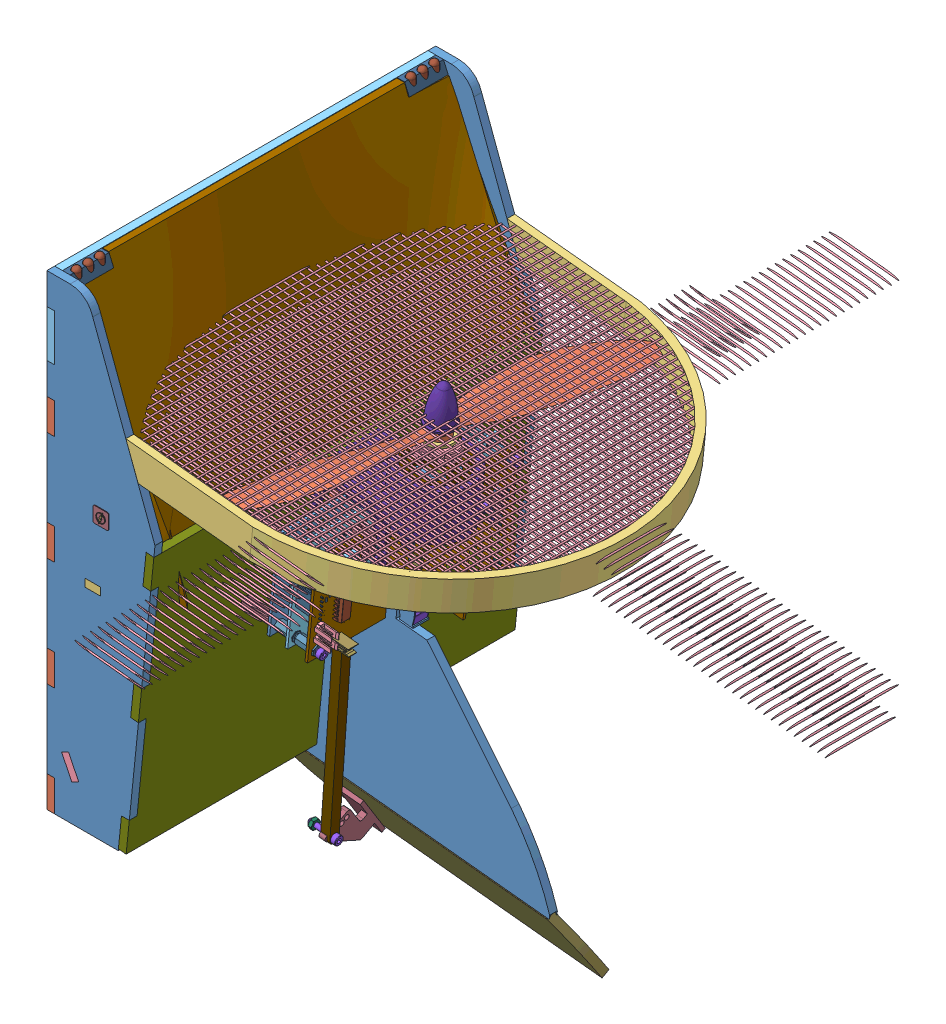
SolidWorks assembly AssTotaleSimu2, configuration Défaut. Lengths in mm. (continued)
Components (placement in the parent): (continued)
- AssStructSimu-1: AssStructSimu [Défaut] at (-125.7658 -1.8483 624.6548) x (1 0 0) z (0 0 -1) size (253.25 324.59 251.6) (continued)
  - AssCarte-1: AssCarte [Défaut] at (38.0121 147.1029 290.772) x (-0.101852 0.9948 0) z (0.9948 0.101852 0) size (66.52 130.57 98.72) (continued)
    - AssEntretoise-3: AssEntretoise [Défaut] at (-106.8199 -51.2976 37.1344) x (0 0 -1) z (1 0 0) size (58.24 7.29 7.81)
      - socket head cap screw 4762_din-1: socket head cap screw 4762_din [EN ISO 4762 M3 x 5 - 5N] at (-2.4967 0.5867 0) size (8 5.5 5.5)
      - hexagonal_spacer_MF_M3_H20_HEX5.5_FTD6_MTL6-1: hexagonal_spacer_MF_M3_H20_HEX5.5_FTD6_MTL6 [Défaut] at (48.3433 0.5867 0) x (0 0 1) z (-1 0 0) size (6.36 5.51 26)
      - hex nut style 1 gradeab_din-1: hex nut style 1 gradeab_din [Hexagon Nut ISO 4032 - M3 - W - N] at (53.3433 0.5867 0) x (0 0.943962 0.330053) z (-1 0 0) size (5.5 6.35 2.4)
      - hexagonal_spacer_MF_M3_H12_HEX5.5_FTD6_MTL6-2: hexagonal_spacer_MF_M3_H12_HEX5.5_FTD6_MTL6 [Défaut] at (27.0633 0.5867 0) x (0 0.248308 0.968681) z (-1 0 0) size (6.36 5.51 18)
      - hexagonal_spacer_MF_M3_H12_HEX5.5_FTD6_MTL6-3: hexagonal_spacer_MF_M3_H12_HEX5.5_FTD6_MTL6 [Défaut] at (13.7833 0.5867 0) x (0 0 1) z (-1 0 0) size (6.36 5.51 18)
    - AssEntretoise-4: AssEntretoise [Défaut] at (-106.8199 68.7024 37.1344) x (0 0 -1) z (1 0 0) size (58.24 7.29 7.81)
      - socket head cap screw 4762_din-1: socket head cap screw 4762_din [EN ISO 4762 M3 x 5 - 5N] at (-2.4967 0.5867 0) size (8 5.5 5.5)
      - hexagonal_spacer_MF_M3_H20_HEX5.5_FTD6_MTL6-1: hexagonal_spacer_MF_M3_H20_HEX5.5_FTD6_MTL6 [Défaut] at (48.3433 0.5867 0) x (0 0 1) z (-1 0 0) size (6.36 5.51 26)
      - hex nut style 1 gradeab_din-1: hex nut style 1 gradeab_din [Hexagon Nut ISO 4032 - M3 - W - N] at (53.3433 0.5867 0) x (0 0.943962 0.330053) z (-1 0 0) size (5.5 6.35 2.4)
      - hexagonal_spacer_MF_M3_H12_HEX5.5_FTD6_MTL6-2: hexagonal_spacer_MF_M3_H12_HEX5.5_FTD6_MTL6 [Défaut] at (27.0633 0.5867 0) x (0 0.248308 0.968681) z (-1 0 0) size (6.36 5.51 18)
      - hexagonal_spacer_MF_M3_H12_HEX5.5_FTD6_MTL6-3: hexagonal_spacer_MF_M3_H12_HEX5.5_FTD6_MTL6 [Défaut] at (13.7833 0.5867 0) x (0 0 1) z (-1 0 0) size (6.36 5.51 18)
    - AssMpu-1: AssMpu [Défaut] at (-150.6881 40.5798 29.6372) x (0.908747 0.417347 0) z (0 0 1) size (8 8 22.28)
      - hex nut style 1 gradeab_din-1: hex nut style 1 gradeab_din [Hexagon Nut ISO 4032 - M3 - W - N] at (0.2783 0.3227 1.2) size (5.5 6.35 2.4)
      - plain washer 6903 type ab_din-1: plain washer 6903 type ab_din [DIN 6903-A3] at (0.2783 0.3227 1.2) x (0 0 1) z (-1 0 0) size (1 8 8)
      - socket head cap screw 4762_din-1: socket head cap screw 4762_din [EN ISO 4762 M3 x 5 - 5N] at (0.2783 0.3227 19.76) x (0 0 -1) z (-0.852155 0.523289 0) size (8 5.5 5.5)
      - hexagonal_spacer_MF_M3_H12_HEX5.5_FTD6_MTL6-1: hexagonal_spacer_MF_M3_H12_HEX5.5_FTD6_MTL6 [Défaut] at (0.2783 0.3227 3.48) size (6.36 5.51 18)
    - AssMpu-2: AssMpu [Défaut] at (-130.3481 40.6665 29.6372) size (8 8 22.28)
      - hex nut style 1 gradeab_din-1: hex nut style 1 gradeab_din [Hexagon Nut ISO 4032 - M3 - W - N] at (0.2783 0.3227 1.2) size (5.5 6.35 2.4)
      - plain washer 6903 type ab_din-1: plain washer 6903 type ab_din [DIN 6903-A3] at (0.2783 0.3227 1.2) x (0 0 1) z (-1 0 0) size (1 8 8)
      - socket head cap screw 4762_din-1: socket head cap screw 4762_din [EN ISO 4762 M3 x 5 - 5N] at (0.2783 0.3227 19.76) x (0 0 -1) z (-0.852155 0.523289 0) size (8 5.5 5.5)
      - hexagonal_spacer_MF_M3_H12_HEX5.5_FTD6_MTL6-1: hexagonal_spacer_MF_M3_H12_HEX5.5_FTD6_MTL6 [Défaut] at (0.2783 0.3227 3.48) size (6.36 5.51 18)
    - AssCosse-1: AssCosse [Défaut] at (-142.6764 26.8797 71.168) x (0 -1 0) z (-0.344896 0 -0.938641) size (9.83 18.66 11.64)
      - socket head cap screw 4762_din-1: socket head cap screw 4762_din [EN ISO 4762 M3 x 6 - 6N] at (-5.1064 0.3659 0) size (9 5.5 5.5)
      - plain washer 6903 type ab_din-1: plain washer 6903 type ab_din [DIN 6903-A3] at (-2.1064 0.3659 0) size (1 8 8)
      - hex nut style 1 gradeab_din-2: hex nut style 1 gradeab_din [Hexagon Nut ISO 4032 - M3 - W - N] at (1.281 0.3659 0) x (0 0.924225 0.381849) z (-1 0 0) size (5.5 6.35 2.4)
      - 31880-1: 31880 [Default] at (0.4936 0.3659 0) x (0 0.344896 -0.938641) z (0 -0.938641 -0.344896) size (5.54 5 17.37)
    - AssCosse-2: AssCosse [Défaut] at (-142.6764 -2.9203 71.168) x (0 -1 0) z (-0.344896 0 -0.938641) size (9.83 18.66 11.64)
      - socket head cap screw 4762_din-1: socket head cap screw 4762_din [EN ISO 4762 M3 x 6 - 6N] at (-5.1064 0.3659 0) size (9 5.5 5.5)
      - plain washer 6903 type ab_din-1: plain washer 6903 type ab_din [DIN 6903-A3] at (-2.1064 0.3659 0) size (1 8 8)
      - hex nut style 1 gradeab_din-2: hex nut style 1 gradeab_din [Hexagon Nut ISO 4032 - M3 - W - N] at (1.281 0.3659 0) x (0 0.924225 0.381849) z (-1 0 0) size (5.5 6.35 2.4)
      - 31880-1: 31880 [Default] at (0.4936 0.3659 0) x (0 0.344896 -0.938641) z (0 -0.938641 -0.344896) size (5.54 5 17.37)
    - AssCosse-3: AssCosse [Défaut] at (-142.6764 12.0797 71.168) x (0 -1 0) z (-0.344896 0 -0.938641) size (9.83 18.66 11.64)
      - socket head cap screw 4762_din-1: socket head cap screw 4762_din [EN ISO 4762 M3 x 6 - 6N] at (-5.1064 0.3659 0) size (9 5.5 5.5)
      - plain washer 6903 type ab_din-1: plain washer 6903 type ab_din [DIN 6903-A3] at (-2.1064 0.3659 0) size (1 8 8)
      - hex nut style 1 gradeab_din-2: hex nut style 1 gradeab_din [Hexagon Nut ISO 4032 - M3 - W - N] at (1.281 0.3659 0) x (0 0.924225 0.381849) z (-1 0 0) size (5.5 6.35 2.4)
      - 31880-1: 31880 [Default] at (0.4936 0.3659 0) x (0 0.344896 -0.938641) z (0 -0.938641 -0.344896) size (5.54 5 17.37)
    - Terminal_QD_Female-1: Terminal_QD_Female [Default] at (-137.2199 31.5422 53.3942) x (0 1 0) z (-1 0 0) size (9.4 5.5 22.35)
    - Terminal_QD_Female-2: Terminal_QD_Female [Default] at (-137.3199 31.5422 36.2942) x (0 -1 0) z (-1 0 0) size (9.4 5.5 22.35)
    - Terminal_QD_Female-3: Terminal_QD_Female [Default] at (-137.2199 1.7422 53.3942) x (0 1 0) z (-1 0 0) size (9.4 5.5 22.35)
    - Terminal_QD_Female-4: Terminal_QD_Female [Default] at (-137.3199 1.7422 35.9942) x (0 1 0) z (-1 0 0) size (9.4 5.5 22.35)
    - Terminal_QD_Female-5: Terminal_QD_Female [Default] at (-137.3199 16.7422 35.9942) x (0 1 0) z (-1 0 0) size (9.4 5.5 22.35)
    - Terminal_QD_Female-6: Terminal_QD_Female [Default] at (-137.2199 16.7422 53.3942) x (0 1 0) z (-1 0 0) size (9.4 5.5 22.35)
- AssTige-1: AssTige [Défaut] at (-241.576 -121.7726 340.4233) x (-0.101791 -0.994204 -0.034587) z (0.9948 -0.101852 0) size (166.39 7.19 19)
  - tige_servo-1: tige_servo [Défaut] at (-106.2712 0.2685 162) size (165 6 6)
  - socket head cap screw 4762_din-2: socket head cap screw 4762_din [EN ISO 4762 M2 x 10 - 10N] at (-104.2712 3.2685 170) x (0 0 -1) z (0.923728 0.383049 0) size (12 3.8 3.8)
  - hex nut style 1 gradeab_din-1: hex nut style 1 gradeab_din [Hexagon Nut ISO 4032 - M3 - W - N] at (55.7288 3.2685 156) size (5.5 6.35 2.4)
  - hex nut style 1 gradeab_din-2: hex nut style 1 gradeab_din [Hexagon Nut ISO 4032 - M2 - W - N] at (-104.2712 3.2685 160) x (0.904801 0.425836 0) z (0 0 1) size (4 4.62 1.6)
  - socket head cap screw 4762_din-3: socket head cap screw 4762_din [EN ISO 4762 M3 x 16 - 16N] at (55.7288 3.2685 171) x (0 0 -1) z (0.923728 0.383049 0) size (19 5.5 5.5)
- AssGoPro-1: AssGoPro [Défaut] at (-119.9926 15.1708 318.2917) x (0 0 -1) z (-0.119031 -0.99289 0) size (64.3 52.3 34.42)
  - GoPRo Frame for LCD Screen-1: GoPRo Frame for LCD Screen [Défaut] at (-2.6935 10.9558 5.5635) size (64.3 47.42 34.42)
    - GoProFrame MJM-1: GoProFrame MJM [Défaut] at (-3.6084 -1.6692 52.45) size (64.3 59.3 23.5)
    - GoPro Hero 3 Front Panel-1: GoPro Hero 3 Front Panel [Défaut] at (-3.6084 -1.6692 55.7) x (-1 0 0) z (0 0 -1) size (59.25 41.2 1.9)
    - GoPro Hero 3 Screen-1: GoPro Hero 3 Screen [Défaut] at (12.7166 3.9308 54.9) size (15 18 1)
    - GoPro Hero 3 Mode Button-1: GoPro Hero 3 Mode Button [Défaut] at (13.4166 -12.4692 54.95) x (-1 0 0) z (0 0 -1) size (11.97 12.11 3.03)
    - GoPro Hero 3 LED Cover-1: GoPro Hero 3 LED Cover [Défaut] at (3.1166 -9.3192 54.85) x (-0.999988 0.004848 0) z (0 0 -1) size (5 5 1.4)
    - GoPro Hero 3 LED Cover-2: GoPro Hero 3 LED Cover [Défaut] at (3.1166 -16.0692 54.85) x (-0.999988 0.004848 0) z (0 0 -1) size (5 5 1.4)
    - GoPro Hero 3 Housing-1: GoPro Hero 3 Housing [Défaut] at (-3.6084 -1.6692 55.7) size (59.37 41.3 29.84)
    - GoPro Hero 3 Lens-1: GoPro Hero 3 Lens [Défaut] at (-18.9334 5.6308 47.35) x (-0.380542 -0.924764 0) z (0 0 -1) size (13.71 15.7 7.94)
    - GoPro Hero 3 Indicator Cover-1: GoPro Hero 3 Indicator Cover [Défaut] at (-25.5834 -22.2692 69.9) x (-0.997412 0 -0.0719) z (0 1 0) size (3 3 2)
    - GoPro Hero 3 Indicator Cover-2: GoPro Hero 3 Indicator Cover [Défaut] at (-28.8834 12.2308 73) x (-0.999992 0.004018 0) z (0 0 1) size (3 3 2)
    - GoPro Hero 3 Indicator Cover-3: GoPro Hero 3 Indicator Cover [Défaut] at (20.6666 16.9308 58.4) x (-0.997739 0 -0.067212) z (0 1 0) size (3 3 2)
    - slot-1: slot [Défaut] at (-24.7434 -9.7363 65.05) x (0 1 0) z (0 0 -1) size (16 15.02 2.44)
    - GoPro Hero 3 HDMI pin-1: GoPro Hero 3 HDMI pin [Défaut] at (-26.982 2.9815 24.7172) x (0.105491 0.98175 -0.158237) z (-0.992872 0.095109 -0.071829) size (3.29 0.86 3.28)
  - support1-2: support1 [Défaut] at (-1.3019 -18.8633 67.0135) x (0 0 1) z (-1 0 0) size (5 5 10)
- AssGouv-1: AssGouv [Défaut] at (-43.2668 -298.2106 479.8345) x (0.9948 -0.101852 0) z (0.055947 0.546439 -0.835628) size (200.18 52.5 43.47)
  - P10_1-1: P10_1 [Défaut] at (-108.1667 -19.4144 197.6829) size (200.18 50.13 5)
  - attache_pale-1: attache_pale [Défaut] at (-49.1667 8.0856 190.1829) x (0 0 -1) z (-1 0 0) size (43.47 35 14)
- Parallax-Servo-Horn-1: Parallax-Servo-Horn [Défaut] at (-69.3162 -29.8353 324.5606) x (0.09792 0.956393 0.27518) z (0.9948 -0.101852 0) size (38.81 38.81 6.17)
- NTM_35-36_engine_assembly-1: NTM_35-36_engine_assembly [Défaut] at (-24.3523 26.8781 325.7101) x (0.9948 -0.101852 0) z (0 0 1) size (60.56 77.2 246.41)
  - engine_base-1: engine_base [Défaut] at (-1.8719 -19.5526 -1.1165) x (0 1 0) z (0 0 1) size (6.8 35 35)
  - engine_bearing-1: engine_bearing [Défaut] at origin size (10 4 10)
  - Propeller_cone-1: Propeller_cone [Défaut] at (-1.8719 33.6474 -4.1165) x (1 0 0) z (0 1 0) size (17.6 17.6 24)
  - engine_bearing-2: engine_bearing [Défaut] at (0 22.8 0) size (10 4 10)
  - NTM_35-36_enginebody-1: NTM_35-36_enginebody [Défaut] at (-1.8719 -12.7526 -1.1165) size (35 31.7 35)
  - Stator-1: Stator [Défaut] at origin size (27.75 22.36 27.94)
  - propellers_10x4-1: propellers_10x4 [Défaut] at (-6.8719 27.4474 -4.9165) size (60.56 10.53 246.41)
  - propeller_washer-1: propeller_washer [Défaut] at (-1.8719 24.4474 -1.1165) x (0 1 0) z (0 0 1) size (2.5 18 18)
  - Propeller_adaptor-1: Propeller_adaptor [Défaut] at (2.1948 17.1101 -3.713) size (23.46 32.5 25)
Mates (geometry in assembly coordinates):
- Coaxiale1: concentric aligned: cylinder of AssStructSimu-1/AssToitMot-1/AssToit-1/P12-1 through (-27.6967 12.5918 324.5936) axis (-0.101852 -0.9948 0) radius 17.5; cylinder of NTM_35-36_engine_assembly-1/NTM_35-36_enginebody-1 through (-25.2217 36.7654 324.5936) axis (-0.101852 -0.9948 0) radius 17.5
- Coïncidente1: coincident anti-aligned: plane of AssStructSimu-1/AssToitMot-1/AssToit-1/P12-1 through (-28.206 7.6178 324.5936) normal (0.101852 0.9948 0); plane of NTM_35-36_engine_assembly-1/engine_bearing-1 through (-28.206 7.6178 324.5936) normal (-0.101852 -0.9948 0)
- Coaxiale2: concentric aligned: cylinder of AssStructSimu-1/AssToitMot-1/AssToit-1/P10_2-1 through (49.7135 -178.7878 324.5936) axis (-0.9948 0.101852 0) radius 2.5; cylinder of AssGouv-1/P10_1-1 through (-94.0351 -164.0702 324.5936) axis (-0.9948 0.101852 0) radius 2.5
- Coïncidente2: coincident aligned: plane of AssStructSimu-1/AssToitMot-1/AssToit-1/P10_2-1 through (-137.5516 -157.1017 322.0936) normal (-0.9948 0.101852 0); plane of AssGouv-1/P10_1-1 through (-137.8791 -160.3008 321.1312) normal (-0.9948 0.101852 0)
- Coaxiale3: concentric aligned: cylinder of AssTige-1/socket head cap screw 4762_din-3 through (-45.5416 -197.7164 335.2292) axis (0.9948 -0.101852 0) radius 1.5; cylinder of AssGouv-1/attache_pale-1 through (-85.9983 -193.5742 335.2292) axis (0.9948 -0.101852 0) radius 1.5
- Coaxiale4: concentric aligned: cylinder of AssStructSimu-1/AssToitMot-1/Parallax-Servo_DUMMY-1 through (-70.6554 -29.6982 324.5606) axis (-0.9948 0.101852 0) radius 2.9845; cylinder of Parallax-Servo-Horn-1 through (-70.6554 -29.6982 324.5606) axis (-0.9948 0.101852 0) radius 2.9845
- Coïncidente3: coincident anti-aligned: plane of AssStructSimu-1/AssToitMot-1/Parallax-Servo_DUMMY-1 through (-74.8246 -29.2713 324.5606) normal (0.9948 -0.101852 0); plane of Parallax-Servo-Horn-1 through (-74.8246 -29.2713 324.5606) normal (-0.9948 0.101852 0)
- Coaxiale5: concentric anti-aligned: cylinder of AssTige-1/socket head cap screw 4762_din-2 through (-30.2498 -38.5418 340.7631) axis (0.9948 -0.101852 0) radius 1; cylinder of Parallax-Servo-Horn-1 through (-69.7931 -34.4932 340.7631) axis (-0.9948 0.101852 0) radius 0.635
- Coïncidente4: coincident anti-aligned: plane of AssTige-1/tige_servo-1 through (-69.6001 -32.608 343.8305) normal (-0.9948 0.101852 0); plane of Parallax-Servo-Horn-1 through (-68.8748 -25.5237 332.3708) normal (0.9948 -0.101852 0)
- Coaxiale6: concentric aligned: cylinder of AssStructSimu-1/AssBase-1/socket head cap screw 4762_din-7 through (-144.5139 -51.9008 369.3436) axis (0 0 1) radius 1.5; cylinder of AssGoPro-1/support1-2 through (-144.5139 -51.9008 319.5936) axis (0 0 1) radius 1.5
- Coïncidente5: coincident anti-aligned: plane of AssStructSimu-1/AssBase-1/support2-1 through (-141.9706 -54.3568 329.5936) normal (0 0 -1); plane of AssGoPro-1/support1-2 through (-146.6985 -49.121 329.5936) normal (0 0 1)
